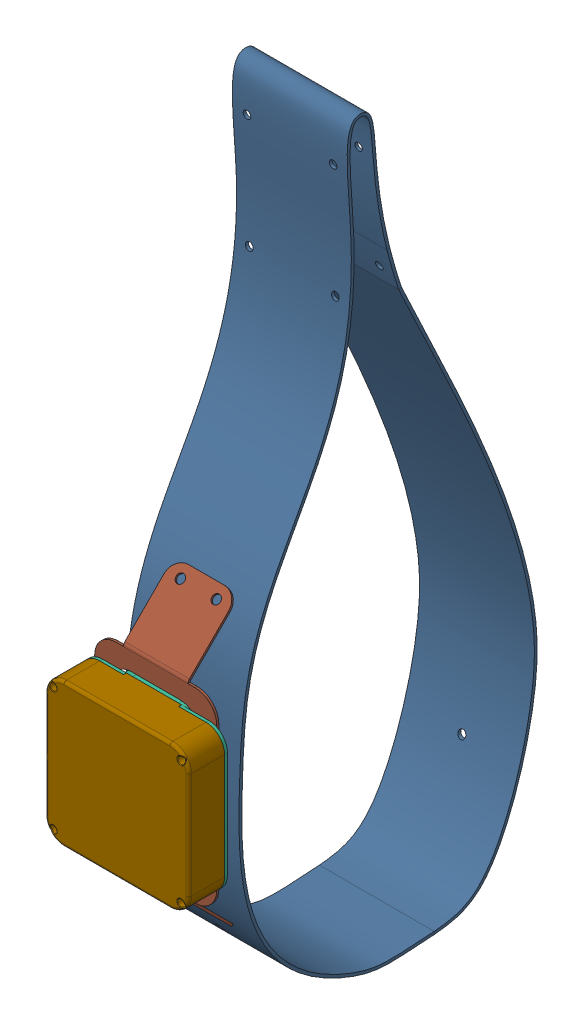
SolidWorks assembly СБ Корпус Peggy Tracker_3, configuration По умолчанию. Lengths in mm.
Overall size (100 542.13 266.88).
305 component instances, 83 part files, 19 mates.
Components (placement in the parent):
- Печатная плата Peggy Tracker-1: Печатная плата Peggy Tracker [По умолчанию] at (-58.3567 -32.1162 37.3232) size (35 62 10.1)
  - Печатная плата Peggy Tracker.step-1: Печатная плата Peggy Tracker.step [Default] at origin size (35 62 10.1)
    - Board.step-1: Board.step [Default] at origin size (35 62 1.56)
      - Open CASCADE STEP translator 6.8 1.1.1.step-1: Open CASCADE STEP translator 6.8 1.1.1.step [Default] at (0 0 -1.5596) size (35 62 1.56)
    - X1.step-1: X1.step [Default] at origin size (28 20 6.7)
      - 6517451856.step-1: 6517451856.step [Default] at (11.15 51.75 6) size (3 3 0.7)
        - Extruded.step-1: Extruded.step [Default] at origin size (3 3 0.7)
      - 6517450176.step-1: 6517450176.step [Default] at (9.1815 45.8445 6) size (6.22 4.19 0.7)
        - Extruded-0.step-1: Extruded-0.step [Default] at origin size (6.22 4.19 0.7)
      - 6517450176.step-2: 6517450176.step [Default] at (9.1815 57.6545 6) size (6.22 4.19 0.7)
        - Extruded-0.step-1: Extruded-0.step [Default] at origin size (6.22 4.19 0.7)
      - 6517449536.step-1: 6517449536.step [Default] at (4.785 51.7495 0) size (2.57 16 6.7)
        - Extruded-1.step-1: Extruded-1.step [Default] at origin size (2.57 16 6.7)
      - 6517449376.step-1: 6517449376.step [Default] at (8.1819 51.7635 6) size (4.22 2.41 0.7)
        - Extruded-2.step-1: Extruded-2.step [Default] at origin size (4.22 2.41 0.7)
      - 6517449056.step-1: 6517449056.step [Default] at (30.8492 51.7495 0) size (1.3 16 6.7)
        - Extruded-3.step-1: Extruded-3.step [Default] at origin size (1.3 16 6.7)
      - 6517448576.step-1: 6517448576.step [Default] at (28.9305 45.5257 6) size (2.54 3.55 0.7)
        - Extruded-4.step-1: Extruded-4.step [Default] at origin size (2.54 3.55 0.7)
      - 6517448256.step-1: 6517448256.step [Default] at (29.4382 51.4325 6) size (1.52 5.71 0.7)
        - Extruded-5.step-1: Extruded-5.step [Default] at origin size (1.52 5.71 0.7)
      - 6517447856.step-1: 6517447856.step [Default] at (18.1354 51.7495 0) size (24.13 16 1)
        - Extruded-6.step-1: Extruded-6.step [Default] at origin size (24.13 16 1)
      - 6517447456.step-1: 6517447456.step [Default] at (18.135 58.925 0) size (24.13 1.65 2.5)
        - Extruded-7.step-1: Extruded-7.step [Default] at origin size (24.13 1.65 2.5)
      - 6517447456.step-2: 6517447456.step [Default] at (18.1356 44.5737 0) size (24.13 1.65 2.5)
        - Extruded-7.step-1: Extruded-7.step [Default] at origin size (24.13 1.65 2.5)
      - 6517447056.step-1: 6517447056.step [Default] at (19.0875 48.7663 0) size (9.53 0.89 2.5)
        - Extruded-8.step-1: Extruded-8.step [Default] at origin size (9.53 0.89 2.5)
      - 6517447056.step-2: 6517447056.step [Default] at (19.0875 54.2273 0) size (9.53 0.89 2.5)
        - Extruded-8.step-1: Extruded-8.step [Default] at origin size (9.53 0.89 2.5)
      - 6517446256.step-1: 6517446256.step [Default] at (28.9302 57.972 6) size (2.54 3.55 0.7)
        - Extruded-9.step-1: Extruded-9.step [Default] at origin size (2.54 3.55 0.7)
      - CircuitWorks-BATT_CR2032.step-1: CircuitWorks-BATT_CR2032.step [Default] at (17.5 51.75 6) x (1 0 0) z (0 1 0) size (20 3.2 20)
    - XW2.step-1: XW2.step [Default] at origin size (2.86 3.01 1.29)
      - IPX.step-1: IPX.step [Default] at (2.0669 38.1281 1.27) x (0 1 0) z (0 0 1) size (3.01 2.86 1.29)
    - XW1.step-1: XW1.step [Default] at origin size (2.86 3.01 1.29)
      - IPX.step-1: IPX.step [Default] at (1.9653 7.4677 1.27) x (0 1 0) z (0 0 1) size (3.01 2.86 1.29)
    - R6.step-1: R6.step [Default] at origin size (0.9 1.7 0.55)
      - 6482559680.step-1: 6482559680.step [Default] at (28.8001 34.2999 0) x (0 -1 0) z (0 0 1) size (1.7 0.9 0.55)
        - Terminal.step-1: Terminal.step [Default] at (-0.85 -0.45 0) size (0.1 0.9 0.55)
          - Open_CASCADE_STEP_translator_6.8_15.2.1.step-1: Open_CASCADE_STEP_translator_6.8_15.2.1.step [Default] at origin size (0.1 0.9 0.55)
        - Terminal.step-2: Terminal.step [Default] at (0.85 0.45 0) x (-1 0 0) z (0 0 1) size (0.1 0.9 0.55)
          - Open_CASCADE_STEP_translator_6.8_15.2.1.step-1: Open_CASCADE_STEP_translator_6.8_15.2.1.step [Default] at origin size (0.1 0.9 0.55)
        - Mid_Body.step-1: Mid_Body.step [Default] at (-0.85 -0.45 0) size (1.59 0.9 0.44)
        - Mark.step-1: Mark.step [Default] at (-0.75 -0.45 0.495) size (1.5 0.9 0.06)
    - X3.step-1: X3.step [Default] at origin size (4.5 5.9 9.4)
      - B2B-PH-K-S(LF)(SN)--3DModel-STEP-56544.step-1: B2B-PH-K-S(LF)(SN)--3DModel-STEP-56544.step [Default] at (32.5449 33.0001 3) x (0 -1 0) z (-1 0 0) size (5.9 9.4 4.5)
    - R5.step-1: R5.step [Default] at origin size (0.95 1.75 0.95)
      - 6482560720.step-1: 6482560720.step [Default] at (27.1578 23.3326 0) x (0 1 0) z (0 0 1) size (1.75 0.95 0.95)
        - Terminal-1.step-1: Terminal-1.step [Default] at (-0.875 -0.475 0) size (0.2 0.95 0.95)
          - Open_CASCADE_STEP_translator_6.8_12.2.1.step-1: Open_CASCADE_STEP_translator_6.8_12.2.1.step [Default] at origin size (0.2 0.95 0.95)
        - Terminal-1.step-2: Terminal-1.step [Default] at (0.875 0.475 0) x (-1 0 0) z (0 0 1) size (0.2 0.95 0.95)
          - Open_CASCADE_STEP_translator_6.8_12.2.1.step-1: Open_CASCADE_STEP_translator_6.8_12.2.1.step [Default] at origin size (0.2 0.95 0.95)
        - Mid_Body-10.step-1: Mid_Body-10.step [Default] at (-0.875 -0.475 0) size (1.56 0.95 0.76)
        - Mark-11.step-1: Mark-11.step [Default] at (-0.675 -0.475 0.855) size (1.35 0.95 0.1)
    - R4.step-1: R4.step [Default] at origin size (0.95 1.75 0.95)
      - 6482560720.step-1: 6482560720.step [Default] at (27.1578 25.8726 0) x (0 1 0) z (0 0 1) size (1.75 0.95 0.95)
        - Terminal-1.step-1: Terminal-1.step [Default] at (-0.875 -0.475 0) size (0.2 0.95 0.95)
          - Open_CASCADE_STEP_translator_6.8_12.2.1.step-1: Open_CASCADE_STEP_translator_6.8_12.2.1.step [Default] at origin size (0.2 0.95 0.95)
        - Terminal-1.step-2: Terminal-1.step [Default] at (0.875 0.475 0) x (-1 0 0) z (0 0 1) size (0.2 0.95 0.95)
          - Open_CASCADE_STEP_translator_6.8_12.2.1.step-1: Open_CASCADE_STEP_translator_6.8_12.2.1.step [Default] at origin size (0.2 0.95 0.95)
        - Mid_Body-10.step-1: Mid_Body-10.step [Default] at (-0.875 -0.475 0) size (1.56 0.95 0.76)
        - Mark-11.step-1: Mark-11.step [Default] at (-0.675 -0.475 0.855) size (1.35 0.95 0.1)
    - R3.step-1: R3.step [Default] at origin size (0.9 1.7 0.55)
      - 6482559680.step-1: 6482559680.step [Default] at (28.8001 31.7999 0) x (0 -1 0) z (0 0 1) size (1.7 0.9 0.55)
        - Terminal.step-1: Terminal.step [Default] at (-0.85 -0.45 0) size (0.1 0.9 0.55)
          - Open_CASCADE_STEP_translator_6.8_15.2.1.step-1: Open_CASCADE_STEP_translator_6.8_15.2.1.step [Default] at origin size (0.1 0.9 0.55)
        - Terminal.step-2: Terminal.step [Default] at (0.85 0.45 0) x (-1 0 0) z (0 0 1) size (0.1 0.9 0.55)
          - Open_CASCADE_STEP_translator_6.8_15.2.1.step-1: Open_CASCADE_STEP_translator_6.8_15.2.1.step [Default] at origin size (0.1 0.9 0.55)
        - Mid_Body.step-1: Mid_Body.step [Default] at (-0.85 -0.45 0) size (1.59 0.9 0.44)
        - Mark.step-1: Mark.step [Default] at (-0.75 -0.45 0.495) size (1.5 0.9 0.06)
    - R2.step-1: R2.step [Default] at origin size (0.9 1.7 0.55)
      - 6482559840.step-1: 6482559840.step [Default] at (24.5109 16.5497 0) x (0 1 0) z (0 0 1) size (1.7 0.9 0.55)
        - Terminal-2.step-1: Terminal-2.step [Default] at (-0.85 -0.45 0) size (0.1 0.9 0.55)
          - Open_CASCADE_STEP_translator_6.8_15.2.1-12.step-1: Open_CASCADE_STEP_translator_6.8_15.2.1-12.step [Default] at origin size (0.1 0.9 0.55)
        - Terminal-2.step-2: Terminal-2.step [Default] at (0.85 0.45 0) x (-1 0 0) z (0 0 1) size (0.1 0.9 0.55)
          - Open_CASCADE_STEP_translator_6.8_15.2.1-12.step-1: Open_CASCADE_STEP_translator_6.8_15.2.1-12.step [Default] at origin size (0.1 0.9 0.55)
        - Mid_Body-13.step-1: Mid_Body-13.step [Default] at (-0.85 -0.45 0) size (1.59 0.9 0.44)
        - Mark-14.step-1: Mark-14.step [Default] at (-0.75 -0.45 0.495) size (1.5 0.9 0.06)
    - R1.step-1: R1.step [Default] at origin size (1.7 0.9 0.55)
      - 6517452256.step-1: 6517452256.step [Default] at (8.2043 34.8489 0) size (1.7 0.9 0.55)
        - Terminal-3.step-1: Terminal-3.step [Default] at (-0.85 -0.45 0) size (0.1 0.9 0.55)
          - Open_CASCADE_STEP_translator_6.8_15.2.1-15.step-1: Open_CASCADE_STEP_translator_6.8_15.2.1-15.step [Default] at origin size (0.1 0.9 0.55)
        - Terminal-3.step-2: Terminal-3.step [Default] at (0.85 0.45 0) x (-1 0 0) z (0 0 1) size (0.1 0.9 0.55)
          - Open_CASCADE_STEP_translator_6.8_15.2.1-15.step-1: Open_CASCADE_STEP_translator_6.8_15.2.1-15.step [Default] at origin size (0.1 0.9 0.55)
        - Mid_Body-16.step-1: Mid_Body-16.step [Default] at (-0.85 -0.45 0) size (1.59 0.9 0.44)
        - Mark-17.step-1: Mark-17.step [Default] at (-0.75 -0.45 0.495) size (1.5 0.9 0.06)
    - L2.step-1: L2.step [Default] at origin size (5.2 5.2 1.8)
      - 6482573440.step-1: 6482573440.step [Default] at (30.1268 13.8076 0.2) x (1 0 0) z (0 -1 0) size (5.2 1.8 5.2)
    - L1.step-1: L1.step [Default] at origin size (0.95 1.75 0.95)
      - 6482561680.step-1: 6482561680.step [Default] at (5.85 37.366 0) x (0 1 0) z (0 0 1) size (1.75 0.95 0.95)
        - Terminal-4.step-1: Terminal-4.step [Default] at (-0.875 -0.475 0) size (1.75 0.95 0.95)
          - Open_CASCADE_STEP_translator_6.8_2.1.1.step-1: Open_CASCADE_STEP_translator_6.8_2.1.1.step [Default] at origin size (0.2 0.95 0.95)
          - Open_CASCADE_STEP_translator_6.8_2.1.2.step-1: Open_CASCADE_STEP_translator_6.8_2.1.2.step [Default] at origin size (0.2 0.95 0.95)
        - Mid_Body-18.step-1: Mid_Body-18.step [Default] at (-0.875 -0.475 0) size (1.35 0.95 0.95)
          - Open_CASCADE_STEP_translator_6.8_2.2.1.step-1: Open_CASCADE_STEP_translator_6.8_2.2.1.step [Default] at origin size (1.35 0.95 0.95)
    - DD2.step-1: DD2.step [Default] at origin size (15 15.5 3.52)
      - 3D_RAK3172.step-1: 3D_RAK3172.step [Default] at (20.536 20.4601 1) x (-1 0 0) z (0 0 1) size (15 15.5 3.52)
        - Board-1.step-1: Board-1.step [Default] at origin size (15 15.5 1.01)
          - Open_CASCADE_STEP_translator_6.8_1.1.1.step-1: Open_CASCADE_STEP_translator_6.8_1.1.1.step [Default] at (0 0 -1.014) size (15 15.5 1.01)
            - Open_CASCADE_STEP_translator_6.8_1.1.1.1.step-1: Open_CASCADE_STEP_translator_6.8_1.1.1.1.step [Default] at origin size (15 15.5 1.01)
        - R11.step-1: R11.step [Default] at origin size (0.6 0.3 0.3)
          - 0201_SMD_Capacitor.step-1: 0201_SMD_Capacitor.step [Default] at (3.4751 6.9342 0.2794) x (-1 0 0) z (0 0 1) size (0.6 0.3 0.3)
        - U2.step-1: U2.step [Default] at origin size (0.99 1.02 0.75)
          - 6590464912.step-1: 6590464912.step [Default] at (5.4483 13.05 0) size (0.99 1.02 0.75)
            - Extruded-19.step-1: Extruded-19.step [Default] at origin size (0.99 1.02 0.75)
        - R4-1.step-1: R4-1.step [Default] at origin size (0.68 0.33 0.34)
          - R0201.step-1: R0201.step [Default] at (3.9176 5.9192 0) x (1 0 0) z (0 -1 0) size (0.68 0.34 0.33)
        - R3-1.step-1: R3-1.step [Default] at origin size (0.33 0.68 0.34)
          - R0201.step-1: R0201.step [Default] at (4.1676 5.6692 0) x (0 1 0) z (1 0 0) size (0.68 0.34 0.33)
        - L2-1.step-1: L2-1.step [Default] at origin size (1.15 0.55 0.41)
          - RES_1005-0402.step-1: RES_1005-0402.step [Default] at (2.2661 6.0198 0) x (1 0 0) z (0 -1 0) size (1.15 0.41 0.55)
        - C10.step-1: C10.step [Default] at origin size (0.6 0.3 0.3)
          - 0201_SMD_Capacitor.step-1: 0201_SMD_Capacitor.step [Default] at (7.1835 13.462 0.2794) x (-1 0 0) z (0 0 1) size (0.6 0.3 0.3)
        - C9.step-1: C9.step [Default] at origin size (0.6 0.3 0.3)
          - 0201_SMD_Capacitor.step-1: 0201_SMD_Capacitor.step [Default] at (7.1835 13.97 0.2794) x (-1 0 0) z (0 0 1) size (0.6 0.3 0.3)
        - C8.step-1: C8.step [Default] at origin size (0.6 0.3 0.3)
          - 0201_SMD_Capacitor.step-1: 0201_SMD_Capacitor.step [Default] at (7.1835 12.954 0.2794) x (-1 0 0) z (0 0 1) size (0.6 0.3 0.3)
        - C7.step-1: C7.step [Default] at origin size (0.6 0.3 0.3)
          - 0201_SMD_Capacitor.step-1: 0201_SMD_Capacitor.step [Default] at (6.0793 11.938 0.2794) x (1 0 0) z (0 0 1) size (0.6 0.3 0.3)
        - C6.step-1: C6.step [Default] at origin size (0.6 0.3 0.3)
          - 0201_SMD_Capacitor.step-1: 0201_SMD_Capacitor.step [Default] at (3.8855 13.5541 0.2794) x (-1 0 0) z (0 0 1) size (0.6 0.3 0.3)
        - CON1.step-1: CON1.step [Default] at origin size (3.4 3.1 1.25)
          - UFL-R-SMD.step-1: UFL-R-SMD.step [Default] at (11.3537 12.7757 0) x (1 0 0) z (0 0 1) size (3.4 3.1 1.25)
            - Part_525.step-1: Part_525.step [Default] at origin size (3 2.6 0.35)
            - Part_739.step-1: Part_739.step [Default] at origin size (2 2 0.9)
            - Part_578.step-1: Part_578.step [Default] at origin size (0.6 0.5 0.1)
            - Part_540.step-1: Part_540.step [Default] at origin size (0.4 1.8 0.1)
            - Part_562.step-1: Part_562.step [Default] at origin size (0.4 1.8 0.1)
            - Part_555.step-1: Part_555.step [Default] at origin size (0.6 0.5 0.1)
        - C4.step-1: C4.step [Default] at origin size (0.6 0.3 0.3)
          - 0201_SMD_Capacitor.step-1: 0201_SMD_Capacitor.step [Default] at (3.7799 9.398 0.2794) x (-1 0 0) z (0 0 1) size (0.6 0.3 0.3)
        - U1.step-1: U1.step [Default] at origin size (7.02 7.02 0.8)
          - QFN48_7x7.step-1: QFN48_7x7.step [Default] at (8.8366 6.9818 0) x (0 1 0) z (1 0 0) size (7.02 0.8 7.02)
        - X1-1.step-1: X1-1.step [Default] at origin size (1.61 2.01 0.71)
          - NT2016SA.step-1: NT2016SA.step [Default] at (1.7496 8.4946 0) x (0 1 0) z (1 0 0) size (2.01 0.71 1.61)
        - C43.step-1: C43.step [Default] at origin size (0.6 0.3 0.3)
          - 0201_SMD_Capacitor.step-1: 0201_SMD_Capacitor.step [Default] at (3.7799 9.9822 0.2794) x (-1 0 0) z (0 0 1) size (0.6 0.3 0.3)
        - C42.step-1: C42.step [Default] at origin size (0.3 0.6 0.3)
          - 0201_SMD_Capacitor.step-1: 0201_SMD_Capacitor.step [Default] at (3.0734 7.9709 0.2794) x (0 -1 0) z (0 0 1) size (0.6 0.3 0.3)
        - R9.step-1: R9.step [Default] at origin size (0.6 0.3 0.3)
          - 0201_SMD_Capacitor.step-1: 0201_SMD_Capacitor.step [Default] at (3.7799 8.8138 0.2794) x (-1 0 0) z (0 0 1) size (0.6 0.3 0.3)
        - C1.step-1: C1.step [Default] at origin size (0.6 0.3 0.3)
          - 0201_SMD_Capacitor.step-1: 0201_SMD_Capacitor.step [Default] at (7.0445 11.557 0.2794) x (1 0 0) z (0 0 1) size (0.6 0.3 0.3)
        - C2.step-1: C2.step [Default] at origin size (0.3 0.6 0.3)
          - 0201_SMD_Capacitor.step-1: 0201_SMD_Capacitor.step [Default] at (7.9756 12.2635 0.2794) x (0 -1 0) z (0 0 1) size (0.6 0.3 0.3)
        - C3.step-1: C3.step [Default] at origin size (0.3 0.6 0.3)
          - 0201_SMD_Capacitor.step-1: 0201_SMD_Capacitor.step [Default] at (2.1844 13.4518 0.2794) x (0 -1 0) z (0 0 1) size (0.6 0.3 0.3)
        - C11.step-1: C11.step [Default] at origin size (0.6 0.3 0.3)
          - 0201_SMD_Capacitor.step-1: 0201_SMD_Capacitor.step [Default] at (1.6623 11.9866 0.2794) x (1 0 0) z (0 0 1) size (0.6 0.3 0.3)
        - C12.step-1: C12.step [Default] at origin size (0.6 0.3 0.3)
          - 0201_SMD_Capacitor.step-1: 0201_SMD_Capacitor.step [Default] at (3.2813 12.573 0.2794) x (1 0 0) z (0 0 1) size (0.6 0.3 0.3)
        - C13.step-1: C13.step [Default] at origin size (0.3 0.6 0.3)
          - 0201_SMD_Capacitor.step-1: 0201_SMD_Capacitor.step [Default] at (4.4958 12.0697 0.2794) x (0 1 0) z (0 0 1) size (0.6 0.3 0.3)
        - C14.step-1: C14.step [Default] at origin size (0.3 0.6 0.3)
          - 0201_SMD_Capacitor.step-1: 0201_SMD_Capacitor.step [Default] at (2.7178 12.6739 0.2794) x (0 -1 0) z (0 0 1) size (0.6 0.3 0.3)
        - C17.step-1: C17.step [Default] at origin size (0.3 0.6 0.3)
          - 0201_SMD_Capacitor.step-1: 0201_SMD_Capacitor.step [Default] at (7.6708 14.4693 0.2794) x (0 -1 0) z (0 0 1) size (0.6 0.3 0.3)
        - C18.step-1: C18.step [Default] at origin size (0.6 0.3 0.3)
          - 0201_SMD_Capacitor.step-1: 0201_SMD_Capacitor.step [Default] at (9.1901 14.1224 0.2794) x (-1 0 0) z (0 0 1) size (0.6 0.3 0.3)
        - C19.step-1: C19.step [Default] at origin size (0.3 0.6 0.3)
          - 0201_SMD_Capacitor.step-1: 0201_SMD_Capacitor.step [Default] at (2.8814 10.8799 0.2794) x (0 1 0) z (0 0 1) size (0.6 0.3 0.3)
        - C22.step-1: C22.step [Default] at origin size (0.3 0.6 0.3)
          - 0201_SMD_Capacitor.step-1: 0201_SMD_Capacitor.step [Default] at (2.0432 11.4801 0.2794) x (0 -1 0) z (0 0 1) size (0.6 0.3 0.3)
        - C21.step-1: C21.step [Default] at origin size (0.3 0.6 0.3)
          - 0201_SMD_Capacitor.step-1: 0201_SMD_Capacitor.step [Default] at (1.5606 11.4801 0.2794) x (0 -1 0) z (0 0 1) size (0.6 0.3 0.3)
        - C23.step-1: C23.step [Default] at origin size (1 0.5 0.5)
          - C0402.step-1: C0402.step [Default] at (8.9644 1.5539 0.254) x (1 0 0) z (0 0 1) size (1 0.5 0.5)
        - C24.step-1: C24.step [Default] at origin size (0.6 0.3 0.3)
          - 0201_SMD_Capacitor.step-1: 0201_SMD_Capacitor.step [Default] at (4.7197 3.8862 0.2794) x (-1 0 0) z (0 0 1) size (0.6 0.3 0.3)
        - C26.step-1: C26.step [Default] at origin size (0.3 0.6 0.3)
          - 0201_SMD_Capacitor.step-1: 0201_SMD_Capacitor.step [Default] at (10.541 2.2265 0.2794) x (0 -1 0) z (0 0 1) size (0.6 0.3 0.3)
        - C44.step-1: C44.step [Default] at origin size (0.6 0.3 0.3)
          - 0201_SMD_Capacitor.step-1: 0201_SMD_Capacitor.step [Default] at (4.7919 9.9822 0.2794) x (-1 0 0) z (0 0 1) size (0.6 0.3 0.3)
        - C29.step-1: C29.step [Default] at origin size (0.6 0.3 0.3)
          - 0201_SMD_Capacitor.step-1: 0201_SMD_Capacitor.step [Default] at (3.9925 7.8486 0.2794) x (1 0 0) z (0 0 1) size (0.6 0.3 0.3)
        - C25.step-1: C25.step [Default] at origin size (0.3 0.6 0.3)
          - 0201_SMD_Capacitor.step-1: 0201_SMD_Capacitor.step [Default] at (10.287 1.6263 0.2794) x (0 1 0) z (0 0 1) size (0.6 0.3 0.3)
        - C31.step-1: C31.step [Default] at origin size (0.6 0.3 0.3)
          - 0201_SMD_Capacitor.step-1: 0201_SMD_Capacitor.step [Default] at (3.9965 7.239 0.2794) x (1 0 0) z (0 0 1) size (0.6 0.3 0.3)
        - C32.step-1: C32.step [Default] at origin size (0.6 0.3 0.3)
          - 0201_SMD_Capacitor.step-1: 0201_SMD_Capacitor.step [Default] at (7.8533 2.3622 0.2794) x (1 0 0) z (0 0 1) size (0.6 0.3 0.3)
        - C33.step-1: C33.step [Default] at origin size (1 0.5 0.5)
          - C0402.step-1: C0402.step [Default] at (5.3048 2.0461 0.254) x (-1 0 0) z (0 0 1) size (1 0.5 0.5)
        - C34.step-1: C34.step [Default] at origin size (0.3 0.6 0.3)
          - 0201_SMD_Capacitor.step-1: 0201_SMD_Capacitor.step [Default] at (4.318 4.2211 0.2794) x (0 1 0) z (0 0 1) size (0.6 0.3 0.3)
        - C35.step-1: C35.step [Default] at origin size (0.6 0.3 0.3)
          - 0201_SMD_Capacitor.step-1: 0201_SMD_Capacitor.step [Default] at (9.0365 2.3622 0.2794) x (1 0 0) z (0 0 1) size (0.6 0.3 0.3)
        - C36.step-1: C36.step [Default] at origin size (0.3 0.6 0.3)
          - 0201_SMD_Capacitor.step-1: 0201_SMD_Capacitor.step [Default] at (13.0302 10.0751 0.2794) x (0 -1 0) z (0 0 1) size (0.6 0.3 0.3)
        - C37.step-1: C37.step [Default] at origin size (0.3 0.6 0.3)
          - 0201_SMD_Capacitor.step-1: 0201_SMD_Capacitor.step [Default] at (3.7338 4.2211 0.2794) x (0 1 0) z (0 0 1) size (0.6 0.3 0.3)
        - C38.step-1: C38.step [Default] at origin size (1 0.5 0.5)
          - C0402.step-1: C0402.step [Default] at (2.3114 4.7323 0.254) x (1 0 0) z (0 0 1) size (1 0.5 0.5)
        - C39.step-1: C39.step [Default] at origin size (0.6 0.3 0.3)
          - 0201_SMD_Capacitor.step-1: 0201_SMD_Capacitor.step [Default] at (4.0593 3.1881 0.2794) x (-1 0 0) z (0 0 1) size (0.6 0.3 0.3)
        - C40.step-1: C40.step [Default] at origin size (0.3 0.6 0.3)
          - 0201_SMD_Capacitor.step-1: 0201_SMD_Capacitor.step [Default] at (3.6576 1.7319 0.2794) x (0 1 0) z (0 0 1) size (0.6 0.3 0.3)
        - L1-1.step-1: L1-1.step [Default] at origin size (0.68 0.33 0.34)
          - R0201.step-1: R0201.step [Default] at (7.8526 11.2014 0) x (-1 0 0) z (0 1 0) size (0.68 0.34 0.33)
        - L3.step-1: L3.step [Default] at origin size (0.33 0.68 0.34)
          - R0201.step-1: R0201.step [Default] at (1.7272 13.1318 0) x (0 -1 0) z (-1 0 0) size (0.68 0.34 0.33)
        - L5.step-1: L5.step [Default] at origin size (0.68 0.33 0.34)
          - R0201.step-1: R0201.step [Default] at (8.0772 13.3096 0) x (-1 0 0) z (0 1 0) size (0.68 0.34 0.33)
        - L6.step-1: L6.step [Default] at origin size (1 0.5 0.5)
          - C0402.step-1: C0402.step [Default] at (5.822 11.0823 0.254) x (1 0 0) z (0 0 1) size (1 0.5 0.5)
        - L7.step-1: L7.step [Default] at origin size (0.68 0.33 0.34)
          - R0201.step-1: R0201.step [Default] at (3.5854 12.1158 0) x (1 0 0) z (0 -1 0) size (0.68 0.34 0.33)
        - L9.step-1: L9.step [Default] at origin size (1.15 0.55 0.41)
          - RES_1005-0402.step-1: RES_1005-0402.step [Default] at (3.9641 11.3538 0) x (-1 0 0) z (0 1 0) size (1.15 0.41 0.55)
        - L20.step-1: L20.step [Default] at origin size (1.6 0.8 0.3)
          - 6559637360.step-1: 6559637360.step [Default] at (12.3698 2.0828 0) x (-1 0 0) z (0 1 0) size (1.6 0.3 0.8)
        - L30.step-1: L30.step [Default] at origin size (1.15 0.55 0.41)
          - RES_1005-0402.step-1: RES_1005-0402.step [Default] at (7.1263 1.8 0) x (-1 0 0) z (0 1 0) size (1.15 0.41 0.55)
        - X2.step-1: X2.step [Default] at origin size (1.2 2 0.61)
          - crystal_rtf2012.step-1: crystal_rtf2012.step [Default] at (2.25 2.8402 0) x (0 1 0) z (1 0 0) size (2 0.61 1.2)
        - R2-1.step-1: R2-1.step [Default] at origin size (0.68 0.33 0.34)
          - R0201.step-1: R0201.step [Default] at (1.9613 10.1854 0) x (1 0 0) z (0 -1 0) size (0.68 0.34 0.33)
        - C5.step-1: C5.step [Default] at origin size (0.6 0.3 0.3)
          - 0201_SMD_Capacitor.step-1: 0201_SMD_Capacitor.step [Default] at (1.8749 6.9342 0.2794) x (-1 0 0) z (0 0 1) size (0.6 0.3 0.3)
        - Free-Models.step-1: Free-Models.step [Default] at origin size (13.4 13.9 2.5)
          - D030A-______.step-1: D030A-______.step [Default] at (2.429 -1.8288 0) size (13.4 13.9 2.5)
    - DD1.step-1: DD1.step [Default] at origin size (9.7 10.1 2.8)
      - 6482566000.step-1: 6482566000.step [Default] at (16.1 34.85 0) x (1 0 0) z (0 0 1) size (9.7 10.1 2.8)
        - Body.step-1: Body.step [Default] at (0 0 0.1) size (9.7 10.1 2.7)
        - Pins.step-1: Pins.step [Default] at origin size (9.56 9.36 0.1)
    - DA1.step-1: DA1.step [Default] at origin size (3 3 1)
      - 6482561360.step-1: 6482561360.step [Default] at (31.2728 20.6686 0) x (0 1 0) z (0 0 1) size (3 3 1)
        - FRAME-DRC0010J.step-1: FRAME-DRC0010J.step [Default] x (1 0 0) z (0 -1 0) size (3 0.2 3)
          - Open CASCADE STEP translator 6.8 1.16.1.2.1.step-1: Open CASCADE STEP translator 6.8 1.16.1.2.1.step [Default] at origin size (1.9 0.2 3)
          - Open CASCADE STEP translator 6.8 1.16.1.2.2.step-1: Open CASCADE STEP translator 6.8 1.16.1.2.2.step [Default] at origin size (0.4 0.2 0.24)
          - Open CASCADE STEP translator 6.8 1.16.1.2.3.step-1: Open CASCADE STEP translator 6.8 1.16.1.2.3.step [Default] at origin size (0.4 0.2 0.24)
          - Open CASCADE STEP translator 6.8 1.16.1.2.4.step-1: Open CASCADE STEP translator 6.8 1.16.1.2.4.step [Default] at origin size (0.4 0.2 0.24)
          - Open CASCADE STEP translator 6.8 1.16.1.2.5.step-1: Open CASCADE STEP translator 6.8 1.16.1.2.5.step [Default] at origin size (0.4 0.2 0.24)
          - Open CASCADE STEP translator 6.8 1.16.1.2.6.step-1: Open CASCADE STEP translator 6.8 1.16.1.2.6.step [Default] at origin size (0.4 0.2 0.24)
          - Open CASCADE STEP translator 6.8 1.16.1.2.7.step-1: Open CASCADE STEP translator 6.8 1.16.1.2.7.step [Default] at origin size (0.4 0.2 0.24)
          - Open CASCADE STEP translator 6.8 1.16.1.2.8.step-1: Open CASCADE STEP translator 6.8 1.16.1.2.8.step [Default] at origin size (0.4 0.2 0.24)
          - Open CASCADE STEP translator 6.8 1.16.1.2.9.step-1: Open CASCADE STEP translator 6.8 1.16.1.2.9.step [Default] at origin size (0.4 0.2 0.24)
          - Open CASCADE STEP translator 6.8 1.16.1.2.10.step-1: Open CASCADE STEP translator 6.8 1.16.1.2.10.step [Default] at origin size (0.4 0.2 0.24)
          - Open CASCADE STEP translator 6.8 1.16.1.2.11.step-1: Open CASCADE STEP translator 6.8 1.16.1.2.11.step [Default] at origin size (0.4 0.2 0.24)
        - BODY-SON.step-1: BODY-SON.step [Default] at (0 0 0.025) x (1 0 0) z (0 -1 0) size (3 0.97 3)
    - C8-1.step-1: C8-1.step [Default] at origin size (1.4 2.15 1.4)
      - 6482573680.step-1: 6482573680.step [Default] at (27.1929 19.9035 0) x (0 -1 0) z (0 0 1) size (2.15 1.4 1.4)
        - Terminal-5.step-1: Terminal-5.step [Default] at (-1.075 -0.7 0) size (2.15 1.4 1.4)
          - Open_CASCADE_STEP_translator_6.8_5.1.1.step-1: Open_CASCADE_STEP_translator_6.8_5.1.1.step [Default] at origin size (0.2 1.4 1.4)
          - Open_CASCADE_STEP_translator_6.8_5.1.2.step-1: Open_CASCADE_STEP_translator_6.8_5.1.2.step [Default] at origin size (0.2 1.4 1.4)
        - Mid_Body-1.step-1: Mid_Body-1.step [Default] at (-1.075 -0.7 0) size (1.75 1.4 1.4)
          - Open_CASCADE_STEP_translator_6.8_5.2.1.step-1: Open_CASCADE_STEP_translator_6.8_5.2.1.step [Default] at origin size (1.75 1.4 1.4)
    - C7-1.step-1: C7-1.step [Default] at origin size (2.1 1.35 1.35)
      - 6482573600.step-1: 6482573600.step [Default] at (31.889 26.8 0) x (1 0 0) z (0 0 1) size (2.1 1.35 1.35)
        - Terminal-6.step-1: Terminal-6.step [Default] at (-1.05 -0.675 0) size (2.1 1.35 1.35)
          - Open_CASCADE_STEP_translator_6.8_24.1.1.step-1: Open_CASCADE_STEP_translator_6.8_24.1.1.step [Default] at origin size (0.2 1.35 1.35)
          - Open_CASCADE_STEP_translator_6.8_24.1.2.step-1: Open_CASCADE_STEP_translator_6.8_24.1.2.step [Default] at origin size (0.2 1.35 1.35)
        - Mid_Body-2.step-1: Mid_Body-2.step [Default] at (-1.05 -0.675 0) size (1.7 1.35 1.35)
          - Open_CASCADE_STEP_translator_6.8_24.2.1.step-1: Open_CASCADE_STEP_translator_6.8_24.2.1.step [Default] at origin size (1.7 1.35 1.35)
    - C6-1.step-1: C6-1.step [Default] at origin size (0.9 1.7 0.9)
      - 6482559520.step-1: 6482559520.step [Default] at (22.727 16.763 0) x (0 -1 0) z (0 0 1) size (1.7 0.9 0.9)
        - Terminal-7.step-1: Terminal-7.step [Default] at (-0.85 -0.45 0) size (1.7 0.9 0.9)
          - Open_CASCADE_STEP_translator_6.8_5.1.1-20.step-1: Open_CASCADE_STEP_translator_6.8_5.1.1-20.step [Default] at origin size (0.2 0.9 0.9)
          - Open_CASCADE_STEP_translator_6.8_5.1.2-21.step-1: Open_CASCADE_STEP_translator_6.8_5.1.2-21.step [Default] at origin size (0.2 0.9 0.9)
        - Mid_Body-3.step-1: Mid_Body-3.step [Default] at (-0.85 -0.45 0) size (1.3 0.9 0.9)
          - Open_CASCADE_STEP_translator_6.8_5.2.1-22.step-1: Open_CASCADE_STEP_translator_6.8_5.2.1-22.step [Default] at origin size (1.3 0.9 0.9)
    - C5-1.step-1: C5-1.step [Default] at origin size (1.35 2.1 1.35)
      - 6482568960.step-1: 6482568960.step [Default] at (24.505 19.939 0) x (0 -1 0) z (0 0 1) size (2.1 1.35 1.35)
        - Terminal-8.step-1: Terminal-8.step [Default] at (-1.05 -0.675 0) size (2.1 1.35 1.35)
          - Open_CASCADE_STEP_translator_6.8_24.1.1-23.step-1: Open_CASCADE_STEP_translator_6.8_24.1.1-23.step [Default] at origin size (0.2 1.35 1.35)
          - Open_CASCADE_STEP_translator_6.8_24.1.2-24.step-1: Open_CASCADE_STEP_translator_6.8_24.1.2-24.step [Default] at origin size (0.2 1.35 1.35)
        - Mid_Body-4.step-1: Mid_Body-4.step [Default] at (-1.05 -0.675 0) size (1.7 1.35 1.35)
          - Open_CASCADE_STEP_translator_6.8_24.2.1-25.step-1: Open_CASCADE_STEP_translator_6.8_24.2.1-25.step [Default] at origin size (1.7 1.35 1.35)
    - C4-1.step-1: C4-1.step [Default] at origin size (0.9 1.7 0.9)
      - 6482559520.step-1: 6482559520.step [Default] at (22.7 19.888 0) x (0 -1 0) z (0 0 1) size (1.7 0.9 0.9)
        - Terminal-7.step-1: Terminal-7.step [Default] at (-0.85 -0.45 0) size (1.7 0.9 0.9)
          - Open_CASCADE_STEP_translator_6.8_5.1.1-20.step-1: Open_CASCADE_STEP_translator_6.8_5.1.1-20.step [Default] at origin size (0.2 0.9 0.9)
          - Open_CASCADE_STEP_translator_6.8_5.1.2-21.step-1: Open_CASCADE_STEP_translator_6.8_5.1.2-21.step [Default] at origin size (0.2 0.9 0.9)
        - Mid_Body-3.step-1: Mid_Body-3.step [Default] at (-0.85 -0.45 0) size (1.3 0.9 0.9)
          - Open_CASCADE_STEP_translator_6.8_5.2.1-22.step-1: Open_CASCADE_STEP_translator_6.8_5.2.1-22.step [Default] at origin size (1.3 0.9 0.9)
    - C3-1.step-1: C3-1.step [Default] at origin size (1.35 2.1 1.35)
      - 6482568960.step-1: 6482568960.step [Default] at (25.7048 39.0008 0) x (0 -1 0) z (0 0 1) size (2.1 1.35 1.35)
        - Terminal-8.step-1: Terminal-8.step [Default] at (-1.05 -0.675 0) size (2.1 1.35 1.35)
          - Open_CASCADE_STEP_translator_6.8_24.1.1-23.step-1: Open_CASCADE_STEP_translator_6.8_24.1.1-23.step [Default] at origin size (0.2 1.35 1.35)
          - Open_CASCADE_STEP_translator_6.8_24.1.2-24.step-1: Open_CASCADE_STEP_translator_6.8_24.1.2-24.step [Default] at origin size (0.2 1.35 1.35)
        - Mid_Body-4.step-1: Mid_Body-4.step [Default] at (-1.05 -0.675 0) size (1.7 1.35 1.35)
          - Open_CASCADE_STEP_translator_6.8_24.2.1-25.step-1: Open_CASCADE_STEP_translator_6.8_24.2.1-25.step [Default] at origin size (1.7 1.35 1.35)
    - C2-1.step-1: C2-1.step [Default] at origin size (0.9 1.7 0.9)
      - 6482561200.step-1: 6482561200.step [Default] at (23.5204 39.0508 0) x (0 1 0) z (0 0 1) size (1.7 0.9 0.9)
        - Terminal-9.step-1: Terminal-9.step [Default] at (-0.85 -0.45 0) size (1.7 0.9 0.9)
          - Open_CASCADE_STEP_translator_6.8_5.1.1-26.step-1: Open_CASCADE_STEP_translator_6.8_5.1.1-26.step [Default] at origin size (0.2 0.9 0.9)
          - Open_CASCADE_STEP_translator_6.8_5.1.2-27.step-1: Open_CASCADE_STEP_translator_6.8_5.1.2-27.step [Default] at origin size (0.2 0.9 0.9)
        - Mid_Body-5.step-1: Mid_Body-5.step [Default] at (-0.85 -0.45 0) size (1.3 0.9 0.9)
          - Open_CASCADE_STEP_translator_6.8_5.2.1-28.step-1: Open_CASCADE_STEP_translator_6.8_5.2.1-28.step [Default] at origin size (1.3 0.9 0.9)
    - C1-1.step-1: C1-1.step [Default] at origin size (0.9 1.7 0.9)
      - 6482559520.step-1: 6482559520.step [Default] at (5.842 33.9488 0) x (0 -1 0) z (0 0 1) size (1.7 0.9 0.9)
        - Terminal-7.step-1: Terminal-7.step [Default] at (-0.85 -0.45 0) size (1.7 0.9 0.9)
          - Open_CASCADE_STEP_translator_6.8_5.1.1-20.step-1: Open_CASCADE_STEP_translator_6.8_5.1.1-20.step [Default] at origin size (0.2 0.9 0.9)
          - Open_CASCADE_STEP_translator_6.8_5.1.2-21.step-1: Open_CASCADE_STEP_translator_6.8_5.1.2-21.step [Default] at origin size (0.2 0.9 0.9)
        - Mid_Body-3.step-1: Mid_Body-3.step [Default] at (-0.85 -0.45 0) size (1.3 0.9 0.9)
          - Open_CASCADE_STEP_translator_6.8_5.2.1-22.step-1: Open_CASCADE_STEP_translator_6.8_5.2.1-22.step [Default] at origin size (1.3 0.9 0.9)
- Case-05-1: Case-05 [По умолчанию] at (-69.8567 1.8838 28.7636) x (0 -1 0) z (0 0 1) size (100 100 21.2)
- Батарейный отсек 2 18650-1: Батарейный отсек 2 18650 [Default] at (-80.8567 -37.1162 49.7636) size (40 78 22)
- Батарейный отсек 2 18650-2: Батарейный отсек 2 18650 [Default] at (-40.8567 -37.1162 49.7636) size (40 78 22)
- Антенна CRJKS0010-LNA-G65U-1: Антенна CRJKS0010-LNA-G65U [По умолчанию] at (-26.3567 5.1418 37.3232) x (-1 0 0) z (0 0 1) size (18 45.5 6.7)
- Case-06-1: Case-06 [По умолчанию] at (-40.8567 -48.1162 73.7636) x (-1 0 0) z (0 0 -1) size (100 100 27.22)
- Ремень-1: Ремень [По умолчанию] at (-40.8567 282.349 -131.1604) x (0 0.995015 0.099729) z (1 0 0) size (523.86 209.36 80.13)
- Металлическое крепление к ошейнику-2: Металлическое крепление к ошейнику [По умолчанию] at (-83.3567 66.8838 46.7636) x (0 -1 0) z (0 0 1) size (203.49 85 36.42)
Mates (geometry in assembly coordinates):
- Coincident1: coincident anti-aligned: plane of Печатная плата Peggy Tracker-1/Печатная плата Peggy Tracker.step-1/Board.step-1/Open CASCADE STEP translator 6.8 1.1.1.step-1 through (-58.3567 -29.1162 35.7636) normal (0 0 -1); plane of Case-05-1 through (-56.3567 -27.1162 35.7636) normal (0 0 1)
- Concentric1: concentric aligned: cylinder of Печатная плата Peggy Tracker-1/Печатная плата Peggy Tracker.step-1/Board.step-1/Open CASCADE STEP translator 6.8 1.1.1.step-1 through (-25.3567 30.8838 35.7636) axis (0 0 -1) radius 1.25; cylinder of Case-05-1 through (-25.3567 30.8838 35.7636) axis (0 0 -1) radius 1.25
- Concentric2: concentric aligned: cylinder of Печатная плата Peggy Tracker-1/Печатная плата Peggy Tracker.step-1/Board.step-1/Open CASCADE STEP translator 6.8 1.1.1.step-1 through (-56.3567 30.8838 35.7636) axis (0 0 -1) radius 1.25; cylinder of Case-05-1 through (-56.3567 30.8838 35.7636) axis (0 0 -1) radius 1.25
- Coincident2: coincident anti-aligned: plane of Батарейный отсек 2 18650-1 through (-40.8567 -37.1162 71.7636) normal (1 0 0); plane of Батарейный отсек 2 18650-2 through (-40.8567 -37.1162 71.7636) normal (-1 0 0)
- Coincident3: coincident aligned: plane of Батарейный отсек 2 18650-1 through (-80.8567 40.8838 71.7636) normal (0 1 0); plane of Батарейный отсек 2 18650-2 through (-40.8567 40.8838 71.7636) normal (0 1 0)
- Coincident4: coincident aligned: plane of Батарейный отсек 2 18650-1 through (-80.8567 -37.1162 49.7636) normal (0 0 -1); plane of Батарейный отсек 2 18650-2 through (-40.8567 -37.1162 49.7636) normal (0 0 -1)
- Coincident5: coincident anti-aligned: plane of Батарейный отсек 2 18650-1 through (-80.8567 -37.1162 71.7636) normal (0 0 1); plane of Case-06-1 through (-40.8567 -48.1162 71.7636) normal (0 0 -1)
- Width1: width aligned: plane of Case-06-1 through (-90.8567 -29.1162 48.7636) normal (-1 0 0); plane of Батарейный отсек 2 18650-1 through (9.1433 -48.1162 48.7636) normal (1 0 0); plane of Case-06-1 through (-80.8567 -37.1162 71.7636) normal (-1 0 0); plane of Батарейный отсек 2 18650-2 through (-0.8567 -37.1162 71.7636) normal (1 0 0)
- Width2: width anti-aligned: plane of Батарейный отсек 2 18650-2 through (-40.8567 40.8838 71.7636) normal (0 1 0); plane of Case-06-1 through (-40.8567 -37.1162 71.7636) normal (0 -1 0); plane of Батарейный отсек 2 18650-2 through (-90.8567 -48.1162 48.7636) normal (0 -1 0); plane of Case-06-1 through (9.1433 51.8838 48.7636) normal (0 1 0)
- Width3: width anti-aligned: plane of Case-06-1 through (-90.8567 -29.1162 48.7636) normal (-1 0 0); plane of Case-05-1 through (9.1433 -48.1162 48.7636) normal (1 0 0); plane of Case-06-1 through (-11.8567 51.8838 46.7636) normal (1 0 0); plane of Case-05-1 through (-69.8567 -48.1162 46.7636) normal (-1 0 0)
- Width4: width anti-aligned: plane of Case-05-1 through (-50.8567 -48.1162 46.7636) normal (0 -1 0); plane of Case-06-1 through (-69.8567 51.8838 46.7636) normal (0 1 0); plane of Case-05-1 through (9.1433 51.8838 48.7636) normal (0 1 0); plane of Case-06-1 through (-90.8567 -48.1162 48.7636) normal (0 -1 0)
- Coincident8: coincident anti-aligned: plane of Печатная плата Peggy Tracker-1/Печатная плата Peggy Tracker.step-1/Board.step-1/Open CASCADE STEP translator 6.8 1.1.1.step-1 through (-58.3567 -29.1162 37.3232) normal (0 0 1); plane of Антенна CRJKS0010-LNA-G65U-1 through (-26.3567 5.1418 37.3232) normal (0 0 -1)
- Distance3: distance = 14 mm aligned: plane of Печатная плата Peggy Tracker-1/Печатная плата Peggy Tracker.step-1/Board.step-1/Open CASCADE STEP translator 6.8 1.1.1.step-1 through (-58.3567 -29.1162 35.7636) normal (-1 0 0); plane of Антенна CRJKS0010-LNA-G65U-1 through (-44.3567 5.1418 41.4732) normal (-1 0 0)
- Distance4: distance = 1.2 mm anti-aligned: plane of Case-05-1 through (-69.8567 1.8838 46.7636) normal (0 0 1); plane of Case-06-1 through (-40.8567 -48.1162 47.9636) normal (0 0 -1)
- Width7: width anti-aligned: plane of Ремень-1 through (-80.8567 -152.8688 -107.5829) normal (-1 0 0); plane of Ремень-1 through (-0.8567 -152.8688 -107.5829) normal (1 0 0); plane of Case-05-1 through (-11.8567 51.8838 46.7636) normal (1 0 0); plane of Case-05-1 through (-69.8567 -48.1162 46.7636) normal (-1 0 0)
- Coincident10: coincident anti-aligned: plane of Case-05-1 through (-56.8567 -35.1162 46.7636) normal (0 0 -1); plane of Металлическое крепление к ошейнику-2 through (-13.3567 51.8838 46.7636) normal (0 0 1)
- Width8: width aligned: plane of Case-05-1 through (-69.8567 -48.1162 46.7636) normal (-1 0 0); plane of Case-05-1 through (-11.8567 51.8838 46.7636) normal (1 0 0); plane of Металлическое крепление к ошейнику-2 through (-83.3567 51.8838 45.2636) normal (-1 0 0); plane of Металлическое крепление к ошейнику-2 through (1.6433 51.8838 45.2636) normal (1 0 0)
- Width9: width aligned: plane of Металлическое крепление к ошейнику-2 through (-68.3567 -63.1162 45.2636) normal (0 -1 0); plane of Металлическое крепление к ошейнику-2 through (-68.3567 66.8838 45.2636) normal (0 1 0); plane of Case-05-1 through (-50.8567 -48.1162 46.7636) normal (0 -1 0); plane of Case-05-1 through (-69.8567 51.8838 46.7636) normal (0 1 0)
- Tangent6: tangent anti-aligned: plane of Case-05-1 through (-69.8567 1.8838 28.7636) normal (0 0 -1); face of Ремень-1
